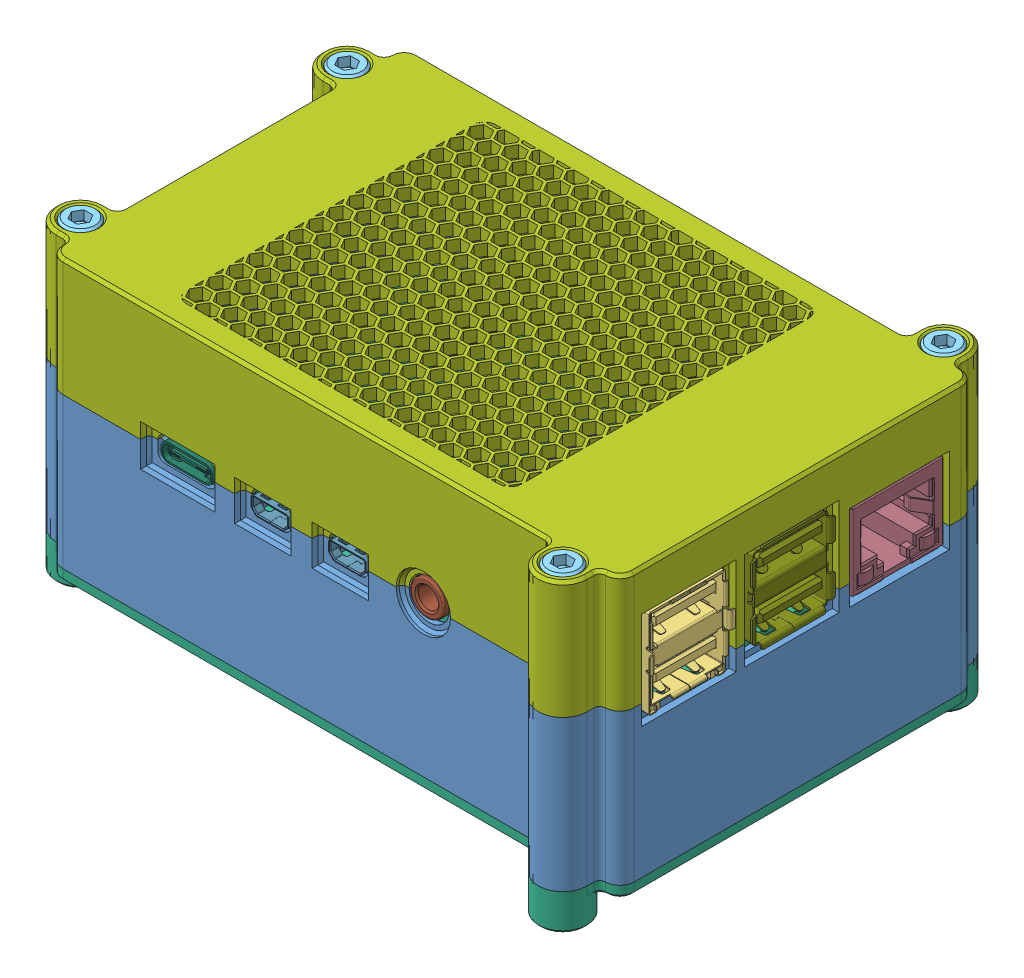
SolidWorks assembly BLOWER, configuration Clean. Lengths in mm.
Overall size (106.79 53.41 74.9).
43 component instances, 25 part files, 47 mates.
Components (placement in the parent):
- BOTTOM-1: BOTTOM [Blank] at (-53.85 -22.79 -31) x (0 0 1) z (-1 0 0) size (74.9 26.3 106.05)
- BAFFLE-1: BAFFLE [Default] at (-0.4852 -20.79 -29) size (44.15 21.79 57.8)
- FAN-1: FAN [Default] at (18.9243 50.309 -15.3439) x (-0.96928 -0.245881 0.006259) z (0.008465 -0.007913 0.999933) size (31.23 8.1 31.18)
  - BLADES-1: BLADES [Default] at (8.6141 60.8719 15.8846) x (0.997386 -0.019795 -0.069495) z (0.069287 -0.011021 0.997536) size (29.14 7.16 29.16)
  - HOUSING-3: HOUSING [Default] at (8.5956 59.9722 15.8759) x (0.99977 -0.020451 -0.006458) z (0.006259 -0.009751 0.999933) size (30 7.03 30)
- socket head cap screw_ai-5: socket head cap screw_ai [HX-SHCS 0.138-32x0.375x0.375-S] at (36.3669 -3.9332 -12) x (0.225951 -0.974139 0) z (0 0 1) size (13.03 5.74 5.74)
- socket head cap screw_ai-6: socket head cap screw_ai [HX-SHCS 0.138-32x0.375x0.375-S] at (12.9875 -9.356 -12) x (0.225951 -0.974139 0) z (0 0 1) size (13.03 5.74 5.74)
- socket head cap screw_ai-7: socket head cap screw_ai [HX-SHCS 0.138-32x0.375x0.375-S] at (36.3669 -3.9332 12) x (0.225951 -0.974139 0) z (0 0 1) size (13.03 5.74 5.74)
- socket head cap screw_ai-8: socket head cap screw_ai [HX-SHCS 0.138-32x0.375x0.375-S] at (12.9875 -9.356 12) x (0.225951 -0.974139 0) z (0 0 1) size (13.03 5.74 5.74)
- BOARD-1: BOARD [Default] at origin size (88.99 19.9 58.4)
  - PCB, RPi4ModelB-1: PCB, RPi4ModelB [Default] at origin size (85 1.6 56)
  - Broadcom BCM2711B0 CPU, RPi4ModelB-1: Broadcom BCM2711B0 CPU, RPi4ModelB [Default] at (-13.25 0.8 -4.5) size (15 2.3 15)
  - 2.54 mm DUPONT MALE PIN HEADER, POE, 2X2, RPi4ModelB-1: 2.54 mm DUPONT MALE PIN HEADER, POE, 2X2, RPi4ModelB [Default] at (19 0.8 -18.5) size (5.08 11.3 5.08)
  - 2.54 mm DUPONT MALE PIN HEADER, IO, 2X20, RPi4ModelB-1: 2.54 mm DUPONT MALE PIN HEADER, IO, 2X20, RPi4ModelB [Default] at (-10 0.8 -24.5) size (50.8 11.3 5.08)
  - Camera Connector, RPi4ModelB-1: Camera Connector, RPi4ModelB [Default] at (4 0.8 16.5) x (0 0 -1) z (1 0 0) size (22.4 5.68 5.07)
  - Microphone Plug, RPi4ModelB-1: Microphone Plug, RPi4ModelB [Default] at (11.5 0.8 21.65) size (7.23 7.55 15)
  - Display Connector, RPi4ModelB-1: Display Connector, RPi4ModelB [Default] at (-38.5 0.8 0) x (0 0 1) z (-1 0 0) size (22.4 5.68 5.07)
  - Gigabit Ethernet Port, RPi4ModelB-1: Gigabit Ethernet Port, RPi4ModelB [Default] at (45.5 7.55 -17.75) x (0 0 -1) z (1 0 0) size (16.2 17.24 21.64)
  - Female Micro HDMI Connector, RPi4ModelB-2: Female Micro HDMI Connector, RPi4ModelB [Default] at (-3 0.8 27.3875) size (6.5 3.51 7.5)
  - Female Micro HDMI Connector, RPi4ModelB-3: Female Micro HDMI Connector, RPi4ModelB [Default] at (-16.5 0.8 27.3875) size (6.5 3.51 7.5)
  - Female USB Type C Connector, RPi4ModelB-1: Female USB Type C Connector, RPi4ModelB [Default] at (-31.3 0.8 26.5419) size (8.94 3.96 7.9)
  - 2X USB3.0 PORTS, RPi4ModelB-2: 2X USB3.0 PORTS, RPi4ModelB [Default] at (37.07 0.8 1) size (17.47 19.41 15.68)
  - 91D77 D9WHV 778K, 4 GB LPDDR4 SDRAM, RPi4ModelB-1: 91D77 D9WHV 778K, 4 GB LPDDR4 SDRAM, RPi4ModelB [Default] at (2.25 0.8 -4.5) size (10 0.8 14.5)
  - Cypress CYW43455 Wireless Module Cover, RPi4ModelB-1: Cypress CYW43455 Wireless Module Cover, RPi4ModelB [Default] at (-30.5 0.8 -14.5) size (11 1.6 13)
  - SD Card Slot, RPi4ModelB-1: SD Card Slot, RPi4ModelB [Default] at (-35.3 -0.8 0) x (0 0 -1) z (-1 0 0) size (11.95 1.45 11.4)
  - VIA VL805 PCIe USB 3.0 controller, RPi4ModelB-1: VIA VL805 PCIe USB 3.0 controller, RPi4ModelB [Default] at (17.5 0.8 4) size (8.8 0.8 8.8)
  - 2X USB2.0 PORTS, RPi4ModelB-1: 2X USB2.0 PORTS, RPi4ModelB [Default] at (37.065 0.65 19) size (17.87 19.16 15.33)
  - Broadcom BCM54213PE Gigabit Ethernet Transceiver, RPi4ModelB-1: Broadcom BCM54213PE Gigabit Ethernet Transceiver, RPi4ModelB [Default] at (16.5 0.8 -10) size (6.8 1 6.8)
  - MxL7704 Universal PMIC, RPi4ModelB-1: MxL7704 Universal PMIC, RPi4ModelB [Default] at (-32.5 0.8 16) size (5.4 0.8 5.4)
- socket head cap screw_ai-1: socket head cap screw_ai [HX-SHCS 0.112-40x0.25x0.25-S] at (-39 3.6348 24.5) x (0 -1 0) z (0 0 -1) size (9.19 4.65 4.65)
- socket head cap screw_ai-4: socket head cap screw_ai [HX-SHCS 0.112-40x0.25x0.25-S] at (-39 3.6348 -24.5) x (0 -1 0) z (0.924225 0 -0.381849) size (9.19 4.65 4.65)
- socket head cap screw_ai-2: socket head cap screw_ai [HX-SHCS 0.112-40x0.25x0.25-S] at (19 3.6348 24.5) x (0 -1 0) z (0 0 -1) size (9.19 4.65 4.65)
- socket head cap screw_ai-3: socket head cap screw_ai [HX-SHCS 0.112-40x0.25x0.25-S] at (19 3.6348 -24.5) x (0 -1 0) z (0 0 -1) size (9.19 4.65 4.65)
- BASE-1: BASE [Clean] at (-53.85 -24.79 -31) x (0 0 1) z (-1 0 0) size (74.9 6.4 106.05)
- socket head cap screw_ai-13: socket head cap screw_ai [HX-SHCS 0.138-32x0.375x0.375-S] at (-56.05 -29.2952 23.25) x (0 1 0) z (0 0 -1) size (13.03 5.74 5.74)
- socket head cap screw_ai-14: socket head cap screw_ai [HX-SHCS 0.138-32x0.375x0.375-S] at (38 -29.2952 33.2) x (0 1 0) z (0 0 -1) size (13.03 5.74 5.74)
- socket head cap screw_ai-15: socket head cap screw_ai [HX-SHCS 0.138-32x0.375x0.375-S] at (-56.05 -29.2952 -23.25) x (0 1 0) z (0 0 -1) size (13.03 5.74 5.74)
- socket head cap screw_ai-16: socket head cap screw_ai [HX-SHCS 0.138-32x0.375x0.375-S] at (38 -29.2952 -33.2) x (0 1 0) z (-0.924225 0 -0.381849) size (13.03 5.74 5.74)
- VENTED-1: VENTED [Clean] at (-53.85 24.01 31) x (0 0 -1) z (-1 0 0) size (74.9 20.5 106.05)
- socket head cap screw_ai-9: socket head cap screw_ai [HX-SHCS 0.138-32x1x1-S] at (-56.05 24.1152 23.25) x (0 -1 0) z (0 0 -1) size (28.91 5.74 5.74)
- socket head cap screw_ai-10: socket head cap screw_ai [HX-SHCS 0.138-32x1x1-S] at (38 24.1152 33.2) x (0 -1 0) z (0 0 -1) size (28.91 5.74 5.74)
- socket head cap screw_ai-11: socket head cap screw_ai [HX-SHCS 0.138-32x1x1-S] at (38 24.1152 -33.2) x (0 -1 0) z (0 0 -1) size (28.91 5.74 5.74)
- socket head cap screw_ai-12: socket head cap screw_ai [HX-SHCS 0.138-32x1x1-S] at (-56.05 24.1152 -23.25) x (0 -1 0) z (0 0 -1) size (28.91 5.74 5.74)
Mates (geometry in assembly coordinates):
- Concentric1: concentric aligned: cylinder of BOARD-1/PCB, RPi4ModelB-1 through (-39 0.8 -24.5) axis (0 1 0) radius 1.35; cylinder of BOTTOM-1 through (-39 -21.79 -24.5) axis (0 1 0) radius 1.4
- Coincident1: coincident anti-aligned: plane of BOARD-1/PCB, RPi4ModelB-1 through (-39 -0.79 24.5) normal (0 -1 0); plane of BOTTOM-1 through (-39 -0.79 24.5) normal (0 1 0)
- Concentric3: concentric aligned: cylinder of BOTTOM-1 through (-39 -21.79 -24.5) axis (0 1 0) radius 1.4; cylinder of socket head cap screw_ai-4 through (-39 35.3848 -24.5) axis (0 1 0) radius 2.3241
- Coincident2: coincident anti-aligned: plane of BOARD-1/PCB, RPi4ModelB-1 through (-39 0.79 -24.5) normal (0 1 0); plane of socket head cap screw_ai-4 through (-39.8875 0.79 -26.648) normal (0 -1 0)
- Concentric4: concentric aligned: cylinder of BOARD-1/PCB, RPi4ModelB-1 through (-39 0.8 24.5) axis (0 1 0) radius 1.35; cylinder of socket head cap screw_ai-1 through (-39 35.3848 24.5) axis (0 1 0) radius 2.3241
- Coincident3: coincident anti-aligned: plane of BOARD-1/PCB, RPi4ModelB-1 through (-39 0.79 24.5) normal (0 1 0); plane of socket head cap screw_ai-1 through (-41.3241 0.79 24.5) normal (0 -1 0)
- Concentric5: concentric aligned: cylinder of BOARD-1/PCB, RPi4ModelB-1 through (19 0.8 -24.5) axis (0 1 0) radius 1.35; cylinder of socket head cap screw_ai-3 through (19 35.3848 -24.5) axis (0 1 0) radius 2.3241
- Coincident4: coincident anti-aligned: plane of BOARD-1/PCB, RPi4ModelB-1 through (19 0.79 -24.5) normal (0 1 0); plane of socket head cap screw_ai-3 through (16.6759 0.79 -24.5) normal (0 -1 0)
- Concentric6: concentric aligned: cylinder of BOARD-1/PCB, RPi4ModelB-1 through (19 0.8 24.5) axis (0 1 0) radius 1.35; cylinder of socket head cap screw_ai-2 through (19 35.3848 24.5) axis (0 1 0) radius 2.3241
- Coincident5: coincident anti-aligned: plane of BOARD-1/PCB, RPi4ModelB-1 through (19 0.79 24.5) normal (0 1 0); plane of socket head cap screw_ai-2 through (16.6759 0.79 24.5) normal (0 -1 0)
- Concentric9: concentric aligned: cylinder of FAN-1/HOUSING-3 through (38.7405 -14.1667 -12) axis (-0.225951 0.974139 0) radius 1.5; cylinder of socket head cap screw_ai-5 through (29.1929 26.9957 -12) axis (-0.225951 0.974139 0) radius 2.8702
- Coincident7: coincident anti-aligned: plane of FAN-1/HOUSING-3 through (12.8054 -12.9965 13) normal (-0.225951 0.974139 0); plane of socket head cap screw_ai-5 through (39.9549 -6.6992 -12) normal (0.225951 -0.974139 0)
- Concentric10: concentric aligned: cylinder of FAN-1/HOUSING-3 through (15.3612 -19.5896 -12) axis (-0.225951 0.974139 0) radius 1.5; cylinder of socket head cap screw_ai-6 through (5.8136 21.5729 -12) axis (-0.225951 0.974139 0) radius 2.8702
- Coincident8: coincident anti-aligned: plane of FAN-1/HOUSING-3 through (12.8054 -12.9965 13) normal (-0.225951 0.974139 0); plane of socket head cap screw_ai-6 through (16.5755 -12.1221 -12) normal (0.225951 -0.974139 0)
- Concentric11: concentric aligned: cylinder of FAN-1/HOUSING-3 through (38.7405 -14.1667 12) axis (-0.225951 0.974139 0) radius 1.5; cylinder of socket head cap screw_ai-7 through (29.1929 26.9957 12) axis (-0.225951 0.974139 0) radius 2.8702
- Coincident9: coincident anti-aligned: plane of FAN-1/HOUSING-3 through (12.8054 -12.9965 13) normal (-0.225951 0.974139 0); plane of socket head cap screw_ai-7 through (39.9549 -6.6992 12) normal (0.225951 -0.974139 0)
- Concentric12: concentric aligned: cylinder of FAN-1/HOUSING-3 through (15.3612 -19.5896 12) axis (-0.225951 0.974139 0) radius 1.5; cylinder of socket head cap screw_ai-8 through (5.8136 21.5729 12) axis (-0.225951 0.974139 0) radius 2.8702
- Coincident10: coincident anti-aligned: plane of FAN-1/HOUSING-3 through (12.8054 -12.9965 13) normal (-0.225951 0.974139 0); plane of socket head cap screw_ai-8 through (16.5755 -12.1221 12) normal (0.225951 -0.974139 0)
- Concentric13: concentric aligned: cylinder of BOTTOM-1 through (38 -22.79 33.2) axis (0 1 0) radius 1.35; cylinder of VENTED-1 through (38 3.51 33.2) axis (0 1 0) radius 1.8
- Concentric14: concentric aligned: cylinder of BOTTOM-1 through (-56.05 -22.79 -23.25) axis (0 1 0) radius 1.35; cylinder of VENTED-1 through (-56.05 3.51 -23.25) axis (0 1 0) radius 1.8
- Coincident11: coincident anti-aligned: plane of BOTTOM-1 through (-51.35 3.51 -28.5) normal (0 1 0); plane of VENTED-1 through (-51.35 3.51 28.5) normal (0 -1 0)
- Concentric15: concentric aligned: cylinder of VENTED-1 through (-56.05 20.61 -23.25) axis (0 1 0) radius 2.9; cylinder of socket head cap screw_ai-12 through (-56.05 55.8652 -23.25) axis (0 1 0) radius 2.8702
- Concentric16: concentric aligned: cylinder of VENTED-1 through (38 20.61 -33.2) axis (0 1 0) radius 2.9; cylinder of socket head cap screw_ai-11 through (38 55.8652 -33.2) axis (0 1 0) radius 2.8702
- Concentric17: concentric aligned: cylinder of VENTED-1 through (38 20.61 33.2) axis (0 1 0) radius 2.9; cylinder of socket head cap screw_ai-10 through (38 55.8652 33.2) axis (0 1 0) radius 2.8702
- Concentric18: concentric aligned: cylinder of VENTED-1 through (-56.05 20.61 23.25) axis (0 1 0) radius 2.9; cylinder of socket head cap screw_ai-9 through (-56.05 55.8652 23.25) axis (0 1 0) radius 2.8702
- Coincident13: coincident anti-aligned: plane of VENTED-1 through (-56.05 20.61 -23.25) normal (0 1 0); plane of socket head cap screw_ai-12 through (-58.9202 20.61 -23.25) normal (0 -1 0)
- Coincident14: coincident anti-aligned: plane of VENTED-1 through (-56.05 20.61 23.25) normal (0 1 0); plane of socket head cap screw_ai-9 through (-58.9202 20.61 23.25) normal (0 -1 0)
- Coincident15: coincident anti-aligned: plane of VENTED-1 through (38 20.61 -33.2) normal (0 1 0); plane of socket head cap screw_ai-11 through (35.1298 20.61 -33.2) normal (0 -1 0)
- Coincident16: coincident anti-aligned: plane of VENTED-1 through (38 20.61 33.2) normal (0 1 0); plane of socket head cap screw_ai-10 through (35.1298 20.61 33.2) normal (0 -1 0)
- Concentric19: concentric aligned: cylinder of BOTTOM-1 through (-56.05 -22.79 -23.25) axis (0 1 0) radius 1.35; cylinder of BASE-1 through (-56.05 -24.79 -23.25) axis (0 1 0) radius 1.8
- Concentric20: concentric aligned: cylinder of BOTTOM-1 through (38 -22.79 -33.2) axis (0 1 0) radius 1.35; cylinder of BASE-1 through (38 -24.79 -33.2) axis (0 1 0) radius 1.8
- Coincident17: coincident anti-aligned: plane of BOTTOM-1 through (-51.35 -22.79 -28.5) normal (0 -1 0); plane of BASE-1 through (-51.35 -22.79 -28.5) normal (0 1 0)
- Concentric21: concentric aligned: cylinder of BASE-1 through (38 -25.79 -33.2) axis (0 -1 0) radius 2.9; cylinder of socket head cap screw_ai-16 through (38 -61.0452 -33.2) axis (0 -1 0) radius 2.8702
- Concentric22: concentric aligned: cylinder of BASE-1 through (-56.05 -25.79 -23.25) axis (0 -1 0) radius 2.9; cylinder of socket head cap screw_ai-15 through (-56.05 -61.0452 -23.25) axis (0 -1 0) radius 2.8702
- Concentric23: concentric aligned: cylinder of BASE-1 through (-56.05 -25.79 23.25) axis (0 -1 0) radius 2.9; cylinder of socket head cap screw_ai-13 through (-56.05 -61.0452 23.25) axis (0 -1 0) radius 2.8702
- Concentric24: concentric aligned: cylinder of BASE-1 through (38 -25.79 33.2) axis (0 -1 0) radius 2.9; cylinder of socket head cap screw_ai-14 through (38 -61.0452 33.2) axis (0 -1 0) radius 2.8702
- Coincident18: coincident anti-aligned: plane of BASE-1 through (38 -25.79 33.2) normal (0 -1 0); plane of socket head cap screw_ai-14 through (40.8702 -25.79 33.2) normal (0 1 0)
- Coincident19: coincident anti-aligned: plane of BASE-1 through (38 -25.79 -33.2) normal (0 -1 0); plane of socket head cap screw_ai-16 through (39.096 -25.79 -35.8527) normal (0 1 0)
- Coincident20: coincident anti-aligned: plane of BASE-1 through (-56.05 -25.79 -23.25) normal (0 -1 0); plane of socket head cap screw_ai-15 through (-53.1798 -25.79 -23.25) normal (0 1 0)
- Coincident21: coincident anti-aligned: plane of BASE-1 through (-56.05 -25.79 23.25) normal (0 -1 0); plane of socket head cap screw_ai-13 through (-53.1798 -25.79 23.25) normal (0 1 0)
- Concentric25: concentric aligned: cylinder of BOARD-1/PCB, RPi4ModelB-1 through (-39 0.8 24.5) axis (0 1 0) radius 1.35; cylinder of BOTTOM-1 through (-39 -21.79 24.5) axis (0 1 0) radius 1.4
- Coincident22: coincident anti-aligned: plane of BOTTOM-1 through (41.75 -7.3094 45.0694) normal (-0.225951 0.974139 0); plane of BAFFLE-1 through (10.4986 -14.5581 29) normal (0.225951 -0.974139 0)
- Coincident25: coincident anti-aligned: plane of BOTTOM-1 through (43.25 -21.79 -28.5) normal (0 1 0); plane of BAFFLE-1 through (-0.4852 -21.79 29) normal (0 -1 0)
- Concentric26: concentric aligned: cylinder of BAFFLE-1 through (40.8627 -23.3159 -12) axis (-0.225951 0.974139 0) radius 1.15; cylinder of FAN-1/HOUSING-3 through (38.7405 -14.1667 -12) axis (-0.225951 0.974139 0) radius 1.5
- Concentric27: concentric aligned: cylinder of BAFFLE-1 through (17.4834 -28.7388 12) axis (-0.225951 0.974139 0) radius 1.15; cylinder of FAN-1/HOUSING-3 through (15.3612 -19.5896 12) axis (-0.225951 0.974139 0) radius 1.5
- Coincident29: coincident anti-aligned: plane of BAFFLE-1 through (14.2897 -19.8381 13.1) normal (-0.225951 0.974139 0); plane of FAN-1/HOUSING-3 through (14.3871 -19.8155 13) normal (0.225951 -0.974139 0)
- Distance2: distance = 0.1 mm anti-aligned: plane of BOTTOM-1 through (-51.35 3.51 29) normal (0 0 -1); plane of BAFFLE-1 through (-0.4852 -22.5772 28.9) normal (0 0 1)
